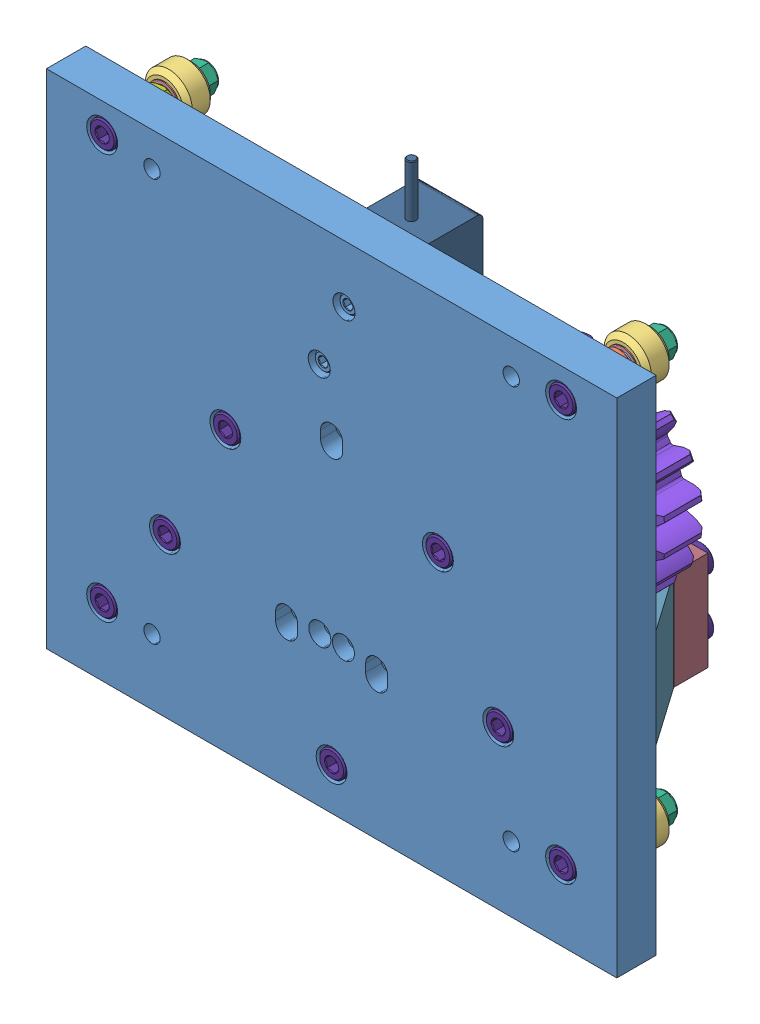
SolidWorks assembly Rudder Pedal Gantry Carriage, configuration Default. Lengths in mm.
Overall size (184.15 170.4 106.96).
90 component instances, 20 part files, 100 mates.
Components (placement in the parent):
- Rudder Pedal Gantry Interface Plate-1: Rudder Pedal Gantry Interface Plate [Default] at (90.01 5647.6627 2781.41) size (184.15 162.18 12.7)
- 819368021615 - Aluminum Spacer 6mm-1: 819368021615 - Aluminum Spacer 6mm [Default] at (74.085 5582.1627 2775.41) x (-1 0 0) z (0 0 1) size (10 10 6)
- 819368020823 - Delrin Mini V Wheel-4: 819368020823 - Delrin Mini V Wheel [Straight] at (74.085 5582.1627 2769.71) x (1 0 0) z (0 -1 0) size (15.23 15.4 15.23)
  - Delrin Mini V Wheel-1: Delrin Mini V Wheel [Default] x (0 -1 0) z (0 0 1) size (8.8 15.23 15.23)
  - Ball Bearing 5 x 10 x 4.2-1: Ball Bearing 5 x 10 x 4.2 [Default] at (0 -2.6 0) x (0 -1 0) z (0.990411 0 0.138155) size (4.2 10 10)
  - Ball Bearing 5 x 10 x 4.2-2: Ball Bearing 5 x 10 x 4.2 [Default] at (0 2.6 0) x (0 1 0) z (-0.887666 0 -0.460488) size (4.2 10 10)
  - Precision Shim 8 x 5 x 1-1: Precision Shim 8 x 5 x 1 [Default] at (0 -0.5 0) x (0.977063 0 -0.212952) z (0.212952 0 0.977063) size (8 1 8)
  - Precision Shim 8 x 5 x 1-2: Precision Shim 8 x 5 x 1 [Default] at (0 4.7 0) x (0.633048 0 -0.774113) z (0.774113 0 0.633048) size (8 1 8)
  - Nylon Insert Lock Nut M5-1: Nylon Insert Lock Nut M5 [Default] at (0 -4.7 0) x (-0.212185 0 -0.97723) z (-0.97723 0 0.212185) size (8 5 9.24)
- 819368021615 - Aluminum Spacer 6mm-2: 819368021615 - Aluminum Spacer 6mm [Default] at (74.085 5452.174 2775.41) x (-0.573309 0.819339 0) z (0 0 1) size (10 10 6)
- 819368020823 - Delrin Mini V Wheel-1: 819368020823 - Delrin Mini V Wheel [Straight] at (74.085 5452.174 2769.71) x (1 0 0) z (0 -1 0) size (15.23 15.4 15.23)
  - Delrin Mini V Wheel-1: Delrin Mini V Wheel [Default] x (0 -1 0) z (0 0 1) size (8.8 15.23 15.23)
  - Ball Bearing 5 x 10 x 4.2-1: Ball Bearing 5 x 10 x 4.2 [Default] at (0 -2.6 0) x (0 -1 0) z (0.990411 0 0.138155) size (4.2 10 10)
  - Ball Bearing 5 x 10 x 4.2-2: Ball Bearing 5 x 10 x 4.2 [Default] at (0 2.6 0) x (0 1 0) z (-0.887666 0 -0.460488) size (4.2 10 10)
  - Precision Shim 8 x 5 x 1-1: Precision Shim 8 x 5 x 1 [Default] at (0 -0.5 0) x (0.977063 0 -0.212952) z (0.212952 0 0.977063) size (8 1 8)
  - Precision Shim 8 x 5 x 1-2: Precision Shim 8 x 5 x 1 [Default] at (0 4.7 0) x (0.633048 0 -0.774113) z (0.774113 0 0.633048) size (8 1 8)
  - Nylon Insert Lock Nut M5-1: Nylon Insert Lock Nut M5 [Default] at (0 -4.7 0) x (-0.212185 0 -0.97723) z (-0.97723 0 0.212185) size (8 5 9.24)
- 819368021011 - Eccentric Spacer 6mm-1: 819368021011 - Eccentric Spacer 6mm [Default] at (-73.351 5581.8705 2781.41) x (0.369816 0.929105 0) z (-0.929105 0.369816 0) size (11.55 8.5 10)
- 819368020823 - Delrin Mini V Wheel-2: 819368020823 - Delrin Mini V Wheel [Straight] at (-74.085 5582.1627 2769.71) x (-1 0 0) z (0 1 0) size (15.23 15.4 15.23)
  - Delrin Mini V Wheel-1: Delrin Mini V Wheel [Default] x (0 -1 0) z (0 0 1) size (8.8 15.23 15.23)
  - Ball Bearing 5 x 10 x 4.2-1: Ball Bearing 5 x 10 x 4.2 [Default] at (0 -2.6 0) x (0 -1 0) z (0.990411 0 0.138155) size (4.2 10 10)
  - Ball Bearing 5 x 10 x 4.2-2: Ball Bearing 5 x 10 x 4.2 [Default] at (0 2.6 0) x (0 1 0) z (-0.887666 0 -0.460488) size (4.2 10 10)
  - Precision Shim 8 x 5 x 1-1: Precision Shim 8 x 5 x 1 [Default] at (0 -0.5 0) x (0.977063 0 -0.212952) z (0.212952 0 0.977063) size (8 1 8)
  - Precision Shim 8 x 5 x 1-2: Precision Shim 8 x 5 x 1 [Default] at (0 4.7 0) x (0.633048 0 -0.774113) z (0.774113 0 0.633048) size (8 1 8)
  - Nylon Insert Lock Nut M5-1: Nylon Insert Lock Nut M5 [Default] at (0 -4.7 0) x (-0.212185 0 -0.97723) z (-0.97723 0 0.212185) size (8 5 9.24)
- 819368021011 - Eccentric Spacer 6mm-2: 819368021011 - Eccentric Spacer 6mm [Default] at (-74.085 5452.174 2781.41) x (-1 0 0) z (0 -1 0) size (11.55 8.5 10)
- 819368020823 - Delrin Mini V Wheel-3: 819368020823 - Delrin Mini V Wheel [Straight] at (-74.085 5452.174 2769.71) x (-1 0 0) z (0 1 0) size (15.23 15.4 15.23)
  - Delrin Mini V Wheel-1: Delrin Mini V Wheel [Default] x (0 -1 0) z (0 0 1) size (8.8 15.23 15.23)
  - Ball Bearing 5 x 10 x 4.2-1: Ball Bearing 5 x 10 x 4.2 [Default] at (0 -2.6 0) x (0 -1 0) z (0.990411 0 0.138155) size (4.2 10 10)
  - Ball Bearing 5 x 10 x 4.2-2: Ball Bearing 5 x 10 x 4.2 [Default] at (0 2.6 0) x (0 1 0) z (-0.887666 0 -0.460488) size (4.2 10 10)
  - Precision Shim 8 x 5 x 1-1: Precision Shim 8 x 5 x 1 [Default] at (0 -0.5 0) x (0.977063 0 -0.212952) z (0.212952 0 0.977063) size (8 1 8)
  - Precision Shim 8 x 5 x 1-2: Precision Shim 8 x 5 x 1 [Default] at (0 4.7 0) x (0.633048 0 -0.774113) z (0.774113 0 0.633048) size (8 1 8)
  - Nylon Insert Lock Nut M5-1: Nylon Insert Lock Nut M5 [Default] at (0 -4.7 0) x (-0.212185 0 -0.97723) z (-0.97723 0 0.212185) size (8 5 9.24)
- GEAR, 3M x 20T x 20PA x 5mm Bore-1: GEAR, 3M x 20T x 20PA x 5mm Bore [Metric - Spur gear 3M 20T 20PA 13FW ---S20O75H20L7N] at (34.31 5519.674 2753.66) x (0 0 -1) z (1 0 0) size (40.75 65.41 65.41)
- GEAR, 3M x 20T x 20PA x 5mm Bore-2: GEAR, 3M x 20T x 20PA x 5mm Bore [Metric - Spur gear 3M 20T 20PA 13FW ---S20O75H20L7N] at (-34.31 5519.674 2753.66) x (0 0 -1) z (1 0 0) size (40.75 65.41 65.41)
- Rudder Pedal Gantry Locking Arm-1: Rudder Pedal Gantry Locking Arm [Default] at (-40.8902 5534.6112 2781.4126) size (85.77 81.54 25.4)
- B14HDP-254-B-4-1: B14HDP-254-B-4 [Default] at (8.6106 5583.123 2781.4126) x (0 0 1) z (0 -1 0) size (26.15 43.85 56.44)
- 1692K230 - SPRING, COMPRESSION, CONFINED SPACE, .60 OD x .625L x 3.57lbs RATE-1: 1692K230 - SPRING, COMPRESSION, CONFINED SPACE, .60 OD x .625L x 3.57lbs RATE [1692K23] at (0 5480.9876 2772.5226) x (0.468976 0 -0.883211) z (0.883211 0 0.468976) size (14.74 6.35 14.56)
- Rudder Pedal Gantry Locking Arm Spring Stop-1: Rudder Pedal Gantry Locking Arm Spring Stop [Default] at (-0.8374 5480.9876 2772.2543) x (-1 0 0) z (0 1 0) size (13.72 15.75 8.89)
- Rudder Carriage Linear Bearing Holder-1: Rudder Carriage Linear Bearing Holder [Default] at (339.725 -1087.7493 -123.7365) size (123.48 58.99 94.03)
  - Rudder Carriage Linear Bearing Holder Lower Shell-1: Rudder Carriage Linear Bearing Holder Lower Shell [Default] at origin size (40 32 10.95)
  - Rudder Carriage Linear Bearing Holder Upper Shell-1: Rudder Carriage Linear Bearing Holder Upper Shell [Default] at origin size (123.48 58.99 77.75)
  - LM8UU v2-1: LM8UU v2 [Default] at (-339.725 6533.262 2827.3504) size (14.96 23.84 14.96)
  - 93625A200 - NUT, M5-0.8, NYLOC, 18-8-1: 93625A200 - NUT, M5-0.8, NYLOC, 18-8 [93625A200] at (-326.725 6524.262 2838.3504) x (-1 0 0) z (0 1 0) size (8 5.15 9.24)
  - 93705A838 - SHCS, M5-0.8 x 30mm, SELF-LOCKING, 18-8-1: 93705A838 - SHCS, M5-0.8 x 30mm, SELF-LOCKING, 18-8 [91292A194] at (-326.725 6524.262 2846.3504) x (0.267759 0.963486 0) z (0 0 1) size (8.5 8.5 35.49)
  - 93625A200 - NUT, M5-0.8, NYLOC, 18-8-2: 93625A200 - NUT, M5-0.8, NYLOC, 18-8 [93625A200] at (-352.725 6524.262 2838.3504) x (-1 0 0) z (0 1 0) size (8 5.15 9.24)
  - 93705A838 - SHCS, M5-0.8 x 30mm, SELF-LOCKING, 18-8-2: 93705A838 - SHCS, M5-0.8 x 30mm, SELF-LOCKING, 18-8 [91292A194] at (-352.725 6524.262 2846.3504) x (0.111609 0.993752 0) z (0 0 1) size (8.5 8.5 35.49)
  - 93625A200 - NUT, M5-0.8, NYLOC, 18-8-3: 93625A200 - NUT, M5-0.8, NYLOC, 18-8 [93625A200] at (-326.725 6542.262 2838.3504) x (-1 0 0) z (0 1 0) size (8 5.15 9.24)
  - 93705A838 - SHCS, M5-0.8 x 30mm, SELF-LOCKING, 18-8-3: 93705A838 - SHCS, M5-0.8 x 30mm, SELF-LOCKING, 18-8 [91292A194] at (-326.725 6542.262 2846.3504) x (-0.015836 0.999875 0) z (0 0 1) size (8.5 8.5 35.49)
  - 93625A200 - NUT, M5-0.8, NYLOC, 18-8-4: 93625A200 - NUT, M5-0.8, NYLOC, 18-8 [93625A200] at (-352.725 6542.262 2838.3504) x (-1 0 0) z (0 1 0) size (8 5.15 9.24)
  - 93705A838 - SHCS, M5-0.8 x 30mm, SELF-LOCKING, 18-8-4: 93705A838 - SHCS, M5-0.8 x 30mm, SELF-LOCKING, 18-8 [91292A194] at (-352.725 6542.262 2846.3504) x (-0.108968 0.994045 0) z (0 0 1) size (8.5 8.5 35.49)
- 93705A838 - SHCS, M5-0.8 x 30mm, SELF-LOCKING, 18-8-1: 93705A838 - SHCS, M5-0.8 x 30mm, SELF-LOCKING, 18-8 [91292A194] at (-34.31 5496.9376 2768.7126) x (-1 0 0.000529) z (0 1 0) size (8.5 8.5 35.49)
- 93625A200 - NUT, M5-0.8, NYLOC, 18-8-1: 93625A200 - NUT, M5-0.8, NYLOC, 18-8 [93625A200] at (-34.31 5478.9696 2768.7126) x (0.99571 0 -0.092533) z (0.092533 0 0.99571) size (8 5.15 9.24)
- 90126A029 - WASHER, .25 x .625, STEEL, ZINC-1: 90126A029 - WASHER, .25 x .625, STEEL, ZINC [90126A029] at (-34.31 5478.9696 2768.7126) x (0 -1 0) z (-0.092533 0 -0.99571) size (2.03 15.88 15.88)
- 93705A838 - SHCS, M5-0.8 x 30mm, SELF-LOCKING, 18-8-2: 93705A838 - SHCS, M5-0.8 x 30mm, SELF-LOCKING, 18-8 [91292A194] at (34.31 5496.9376 2768.7126) x (0.981982 0 -0.188974) z (0 1 0) size (8.5 8.5 35.49)
- 93625A200 - NUT, M5-0.8, NYLOC, 18-8-2: 93625A200 - NUT, M5-0.8, NYLOC, 18-8 [93625A200] at (34.31 5478.9696 2768.7126) x (-0.982082 0 0.188455) z (-0.188455 0 -0.982082) size (8 5.15 9.24)
- 90126A029 - WASHER, .25 x .625, STEEL, ZINC-2: 90126A029 - WASHER, .25 x .625, STEEL, ZINC [90126A029] at (34.31 5478.9696 2768.7126) x (0 -1 0) z (0.188455 0 0.982082) size (2.03 15.88 15.88)
- 93705A838 - SHCS, M5-0.8 x 30mm, SELF-LOCKING, 18-8-3: 93705A838 - SHCS, M5-0.8 x 30mm, SELF-LOCKING, 18-8 [91292A194] at (-34.31 5519.674 2759.11) x (-1 0.000529 0) z (0 0 -1) size (8.5 8.5 35.49)
- 93625A200 - NUT, M5-0.8, NYLOC, 18-8-3: 93625A200 - NUT, M5-0.8, NYLOC, 18-8 [93625A200] at (-34.31 5519.674 2765.11) x (0.973495 -0.228707 0) z (0.228707 0.973495 0) size (8 5.15 9.24)
- 90126A029 - WASHER, .25 x .625, STEEL, ZINC-3: 90126A029 - WASHER, .25 x .625, STEEL, ZINC [90126A029] at (-34.31 5519.674 2767.142) x (0 0 -1) z (-0.092533 0.99571 0) size (2.03 15.88 15.88)
- 93705A838 - SHCS, M5-0.8 x 30mm, SELF-LOCKING, 18-8-4: 93705A838 - SHCS, M5-0.8 x 30mm, SELF-LOCKING, 18-8 [91292A194] at (34.31 5519.674 2759.11) x (-0.987434 -0.158031 0) z (0 0 -1) size (8.5 8.5 35.49)
- 93625A200 - NUT, M5-0.8, NYLOC, 18-8-4: 93625A200 - NUT, M5-0.8, NYLOC, 18-8 [93625A200] at (34.31 5519.674 2765.11) x (0.997443 -0.071464 0) z (0.071464 0.997443 0) size (8 5.15 9.24)
- 90126A029 - WASHER, .25 x .625, STEEL, ZINC-4: 90126A029 - WASHER, .25 x .625, STEEL, ZINC [90126A029] at (34.31 5519.674 2767.142) x (0 0 -1) z (-0.249235 0.968443 0) size (2.03 15.88 15.88)
- Ball Bearing 5 x 10 x 4.2-1: Ball Bearing 5 x 10 x 4.2 [Default] at (34.31 5519.674 2778.5139) x (0 0 1) z (-0.998847 0.048007 0) size (4.2 10 10)
- Ball Bearing 5 x 10 x 4.2-2: Ball Bearing 5 x 10 x 4.2 [Default] at (-34.31 5519.674 2778.5139) x (0 0 1) z (-0.617174 -0.786826 0) size (4.2 10 10)
- 93705A838 - SHCS, M5-0.8 x 30mm, SELF-LOCKING, 18-8-6: 93705A838 - SHCS, M5-0.8 x 30mm, SELF-LOCKING, 18-8 [91292A194] at (-53.8009 5480.5627 2759.11) x (0.987434 0.158031 0) z (0 0 -1) size (8.5 8.5 35.49)
- 90126A029 - WASHER, .25 x .625, STEEL, ZINC-6: 90126A029 - WASHER, .25 x .625, STEEL, ZINC [90126A029] at (-53.8009 5480.5627 2771.885) x (0 0 -1) z (0.249235 -0.968443 0) size (2.03 15.88 15.88)
- 93625A200 - NUT, M5-0.8, NYLOC, 18-8-6: 93625A200 - NUT, M5-0.8, NYLOC, 18-8 [93625A200] at (-53.8009 5480.5627 2769.853) x (-0.99742 0.071781 0) z (-0.071781 -0.99742 0) size (8 5.15 9.24)
- 93705A838 - SHCS, M5-0.8 x 30mm, SELF-LOCKING, 18-8-7: 93705A838 - SHCS, M5-0.8 x 30mm, SELF-LOCKING, 18-8 [91292A194] at (0 5443.1314 2759.11) x (0.949887 0.312592 0) z (0 0 -1) size (8.5 8.5 35.49)
- 90126A029 - WASHER, .25 x .625, STEEL, ZINC-7: 90126A029 - WASHER, .25 x .625, STEEL, ZINC [90126A029] at (0 5443.1314 2771.885) x (0 0 -1) z (0.399631 -0.916676 0) size (2.03 15.88 15.88)
- 93625A200 - NUT, M5-0.8, NYLOC, 18-8-7: 93625A200 - NUT, M5-0.8, NYLOC, 18-8 [93625A200] at (0 5443.1314 2769.853) x (-0.996185 -0.087271 0) z (0.087271 -0.996185 0) size (8 5.15 9.24)
- 93705A838 - SHCS, M5-0.8 x 30mm, SELF-LOCKING, 18-8-9: 93705A838 - SHCS, M5-0.8 x 30mm, SELF-LOCKING, 18-8 [91292A194] at (53.8009 5480.5627 2759.11) x (0.902352 0.430999 0) z (0 0 -1) size (8.5 8.5 35.49)
- 90126A029 - WASHER, .25 x .625, STEEL, ZINC-9: 90126A029 - WASHER, .25 x .625, STEEL, ZINC [90126A029] at (53.8009 5480.5627 2771.885) x (0 0 -1) z (0.513101 -0.858328 0) size (2.03 15.88 15.88)
- 93625A200 - NUT, M5-0.8, NYLOC, 18-8-9: 93625A200 - NUT, M5-0.8, NYLOC, 18-8 [93625A200] at (53.8009 5480.5627 2769.853) x (-0.976963 -0.213407 0) z (0.213407 -0.976963 0) size (8 5.15 9.24)
- 93705A838 - SHCS, M5-0.8 x 30mm, SELF-LOCKING, 18-8-11: 93705A838 - SHCS, M5-0.8 x 30mm, SELF-LOCKING, 18-8 [91292A194] at (-74.085 5582.1627 2759.11) x (0.902352 0.430999 0) z (0 0 -1) size (8.5 8.5 35.49)
- 93705A838 - SHCS, M5-0.8 x 30mm, SELF-LOCKING, 18-8-12: 93705A838 - SHCS, M5-0.8 x 30mm, SELF-LOCKING, 18-8 [91292A194] at (-74.085 5451.384 2759.11) x (0.822602 0.568618 0) z (0 0 -1) size (8.5 8.5 35.49)
- 93705A838 - SHCS, M5-0.8 x 30mm, SELF-LOCKING, 18-8-14: 93705A838 - SHCS, M5-0.8 x 30mm, SELF-LOCKING, 18-8 [91292A194] at (74.085 5452.174 2759.11) x (0.743503 0.668733 0) z (0 0 -1) size (8.5 8.5 35.49)
- 93705A838 - SHCS, M5-0.8 x 30mm, SELF-LOCKING, 18-8-16: 93705A838 - SHCS, M5-0.8 x 30mm, SELF-LOCKING, 18-8 [91292A194] at (74.085 5582.1627 2759.11) x (0.677932 0.735125 0) z (0 0 -1) size (8.5 8.5 35.49)
- 91251A146 - SHCS, 6-32 X .375, STEEL, BLACK-OXIDE-1: 91251A146 - SHCS, 6-32 X .375, STEEL, BLACK-OXIDE [91251A146] at (4 5573.123 2779.8098) x (0.923728 0.383049 0) z (0 0 -1) size (5.74 5.74 13.47)
- 91251A146 - SHCS, 6-32 X .375, STEEL, BLACK-OXIDE-2: 91251A146 - SHCS, 6-32 X .375, STEEL, BLACK-OXIDE [91251A146] at (-4 5553.123 2779.8098) x (0.923728 0.383049 0) z (0 0 -1) size (5.74 5.74 13.47)
- 91251A146 - SHCS, 6-32 X .375, STEEL, BLACK-OXIDE-3: 91251A146 - SHCS, 6-32 X .375, STEEL, BLACK-OXIDE [91251A146] at (-3.81 5477.8126 2777.2698) x (0.923728 0.383049 0) z (0 0 -1) size (5.74 5.74 13.47)
- 91251A146 - SHCS, 6-32 X .375, STEEL, BLACK-OXIDE-4: 91251A146 - SHCS, 6-32 X .375, STEEL, BLACK-OXIDE [91251A146] at (3.81 5477.8126 2777.2698) x (0.923728 0.383049 0) z (0 0 -1) size (5.74 5.74 13.47)
- 91251A146 - SHCS, 6-32 X .375, STEEL, BLACK-OXIDE-5: 91251A146 - SHCS, 6-32 X .375, STEEL, BLACK-OXIDE [91251A146] at (-14.5414 5476.9439 2777.2698) x (0.216826 -0.97621 0) z (0 0 -1) size (5.74 5.74 13.47)
- 91251A146 - SHCS, 6-32 X .375, STEEL, BLACK-OXIDE-7: 91251A146 - SHCS, 6-32 X .375, STEEL, BLACK-OXIDE [91251A146] at (14.5414 5476.9439 2777.2698) x (0.044015 -0.999031 0) z (0 0 -1) size (5.74 5.74 13.47)
- 91251A146 - SHCS, 6-32 X .375, STEEL, BLACK-OXIDE-9: 91251A146 - SHCS, 6-32 X .375, STEEL, BLACK-OXIDE [91251A146] at (0 5534.964 2777.2698) x (-0.130134 -0.991496 0) z (0 0 -1) size (5.74 5.74 13.47)
- 93365A130 - INSERT, 6-32, BRASS, FOR PLASTICS-2: 93365A130 - INSERT, 6-32, BRASS, FOR PLASTICS [93365A130] at (-14.5414 5476.9439 2781.4126) x (-0.85131 -0.524663 0) z (-0.524663 0.85131 0) size (5.56 4.29 5.56)
- 93365A130 - INSERT, 6-32, BRASS, FOR PLASTICS-4: 93365A130 - INSERT, 6-32, BRASS, FOR PLASTICS [93365A130] at (14.5414 5476.9439 2781.4126) x (-0.777574 -0.628792 0) z (-0.628792 0.777574 0) size (5.56 4.29 5.56)
- 93365A130 - INSERT, 6-32, BRASS, FOR PLASTICS-6: 93365A130 - INSERT, 6-32, BRASS, FOR PLASTICS [93365A130] at (-3.81 5477.8126 2781.4126) x (-0.715577 -0.698533 0) z (-0.698533 0.715577 0) size (5.56 4.29 5.56)
- 93365A130 - INSERT, 6-32, BRASS, FOR PLASTICS-8: 93365A130 - INSERT, 6-32, BRASS, FOR PLASTICS [93365A130] at (3.81 5477.8126 2781.4126) x (-0.676489 -0.736453 0) z (-0.736453 0.676489 0) size (5.56 4.29 5.56)
- 93365A130 - INSERT, 6-32, BRASS, FOR PLASTICS-1: 93365A130 - INSERT, 6-32, BRASS, FOR PLASTICS [93365A130] at (0 5534.964 2781.4126) x (-0.923728 -0.383049 0) z (-0.383049 0.923728 0) size (5.56 4.29 5.56)
Mates (geometry in assembly coordinates):
- Concentric67: concentric: cylinder of 819368020823 - Delrin Mini V Wheel-4/Precision Shim 8 x 5 x 1-2 through (74.085 5582.1627 2775.41) axis (0 0 -1) radius 4; cylinder of 819368021615 - Aluminum Spacer 6mm-1 through (74.085 5582.1627 2781.41) axis (0 0 -1) radius 5
- Coincident356: coincident: plane of 819368020823 - Delrin Mini V Wheel-4/Precision Shim 8 x 5 x 1-2 through (74.085 5582.1627 2775.41) normal (0 0 1); plane of 819368021615 - Aluminum Spacer 6mm-1 through (74.085 5582.1627 2775.41) normal (0 0 -1)
- Coincident358: coincident: plane of Rudder Pedal Gantry Interface Plate-1 through (90.01 5647.6627 2781.41) normal (0 0 -1); plane of 819368021615 - Aluminum Spacer 6mm-1 through (74.085 5582.1627 2781.41) normal (0 0 1)
- Distance9: distance = 9.525 mm: plane of 819368021615 - Aluminum Spacer 6mm-1 through (74.085 5582.1627 2775.41) normal (0 -1 0); plane of Rudder Pedal Gantry Interface Plate-1 through (92.075 5591.6877 2794.11) normal (0 1 0)
- Coincident359: coincident: plane of 819368020823 - Delrin Mini V Wheel-4 through (74.085 5582.1627 2769.71) normal (0 0 1); plane of 819368020823 - Delrin Mini V Wheel-1 through (74.085 5452.174 2769.71) normal (0 0 1)
- Coincident360: coincident: plane of 819368020823 - Delrin Mini V Wheel-4 through (74.085 5582.1627 2769.71) normal (1 0 0); plane of 819368020823 - Delrin Mini V Wheel-1 through (74.085 5452.174 2769.71) normal (1 0 0)
- Concentric68: concentric: cylinder of 819368020823 - Delrin Mini V Wheel-1/Precision Shim 8 x 5 x 1-2 through (74.085 5452.174 2775.41) axis (0 0 -1) radius 4; cylinder of 819368021615 - Aluminum Spacer 6mm-2 through (74.085 5452.174 2781.41) axis (0 0 -1) radius 5
- Coincident361: coincident: plane of 819368020823 - Delrin Mini V Wheel-1/Precision Shim 8 x 5 x 1-2 through (74.085 5452.174 2775.41) normal (0 0 1); plane of 819368021615 - Aluminum Spacer 6mm-2 through (74.085 5452.174 2775.41) normal (0 0 -1)
- Concentric70: concentric aligned: cylinder of 819368020823 - Delrin Mini V Wheel-2/Precision Shim 8 x 5 x 1-2 through (-74.085 5582.1627 2775.41) axis (0 0 -1) radius 4; cylinder of 819368021011 - Eccentric Spacer 6mm-1 through (-74.085 5582.1627 2783.91) axis (0 0 -1) radius 2.5
- Coincident362: coincident anti-aligned: plane of 819368020823 - Delrin Mini V Wheel-2/Precision Shim 8 x 5 x 1-2 through (-74.085 5582.1627 2775.41) normal (0 0 1); circle of 819368021011 - Eccentric Spacer 6mm-1
- Concentric71: concentric aligned: cylinder of 819368020823 - Delrin Mini V Wheel-3/Delrin Mini V Wheel-1 through (-74.085 5452.174 2769.71) axis (0 0 -1) radius 7.615; cylinder of 819368021011 - Eccentric Spacer 6mm-2 through (-74.085 5452.174 2783.91) axis (0 0 -1) radius 3.555
- Coincident363: coincident anti-aligned: plane of 819368020823 - Delrin Mini V Wheel-3/Precision Shim 8 x 5 x 1-2 through (-74.085 5452.174 2775.41) normal (0 0 1); circle of 819368021011 - Eccentric Spacer 6mm-2
- Parallel3: parallel aligned: plane of GEAR, 3M x 20T x 20PA x 5mm Bore-1 through (34.31 5519.674 2781.4139) normal (0 0 1); plane of Rudder Pedal Gantry Locking Arm-1 through (-40.8902 5534.6112 2781.4126) normal (0 0 1)
- Coincident414: coincident: cone of GEAR, 3M x 20T x 20PA x 5mm Bore-2 through (-34.31 5497.235 2768.7139) axis (0 1 0); circle of 93705A838 - SHCS, M5-0.8 x 30mm, SELF-LOCKING, 18-8-1
- Tangent18: tangent anti-aligned: cylinder of GEAR, 3M x 20T x 20PA x 5mm Bore-2 through (-34.31 5519.674 2781.4139) axis (0 0 -1) radius 26.249; plane of B14HDP-254-B-4-1 through (10 5545.923 2757.2626) normal (0 -1 0)
- Concentric82: concentric anti-aligned: cylinder of Rudder Pedal Gantry Locking Arm-1 through (-34.31 5461.9376 2768.7126) axis (0 -1 0) radius 2.75; cylinder of 93705A838 - SHCS, M5-0.8 x 30mm, SELF-LOCKING, 18-8-1 through (-34.31 5466.9376 2768.7126) axis (0 1 0) radius 2.5
- Coincident405: coincident anti-aligned: plane of Rudder Pedal Gantry Locking Arm-1 through (-31.56 5466.9376 2768.7126) normal (0 -1 0); plane of 93705A838 - SHCS, M5-0.8 x 30mm, SELF-LOCKING, 18-8-1 through (-34.31 5466.9376 2768.7126) normal (0 1 0)
- Coincident406: coincident: plane of assembly; plane of Rudder Pedal Gantry Locking Arm-1 through (50.8 5476.9376 2756.0126) normal (0 1 0); plane of 90126A029 - WASHER, .25 x .625, STEEL, ZINC-1 through (-34.31 5476.9376 2768.7126) normal (0 -1 0)
- Concentric87: concentric anti-aligned: cylinder of Rudder Pedal Gantry Locking Arm-1 through (34.31 5461.9376 2768.7126) axis (0 -1 0) radius 2.75; cylinder of 93705A838 - SHCS, M5-0.8 x 30mm, SELF-LOCKING, 18-8-2 through (34.31 5466.9376 2768.7126) axis (0 1 0) radius 2.5
- Coincident409: coincident anti-aligned: plane of Rudder Pedal Gantry Locking Arm-1 through (37.06 5466.9376 2768.7126) normal (0 -1 0); plane of 93705A838 - SHCS, M5-0.8 x 30mm, SELF-LOCKING, 18-8-2 through (34.31 5466.9376 2768.7126) normal (0 1 0)
- Coincident410: coincident: plane of assembly; plane of Rudder Pedal Gantry Locking Arm-1 through (50.8 5476.9376 2756.0126) normal (0 1 0); plane of 90126A029 - WASHER, .25 x .625, STEEL, ZINC-2 through (34.31 5476.9376 2768.7126) normal (0 -1 0)
- Coincident418: coincident anti-aligned: plane of Rudder Pedal Gantry Locking Arm-1 through (0 5487.3376 2790.3026) normal (0 -1 0); plane of 1692K230 - SPRING, COMPRESSION, CONFINED SPACE, .60 OD x .625L x 3.57lbs RATE-1 through (0 5487.3376 2772.5226) normal (0 1 0)
- Concentric93: concentric anti-aligned: cylinder of Rudder Pedal Gantry Locking Arm-1 through (0 5487.3376 2772.5226) axis (0 -1 0) radius 7.62; circle of 1692K230 - SPRING, COMPRESSION, CONFINED SPACE, .60 OD x .625L x 3.57lbs RATE-1
- Coincident425: coincident aligned: plane of Rudder Pedal Gantry Locking Arm-1 through (-40.8902 5534.6112 2781.4126) normal (0 0 1); plane of Rudder Pedal Gantry Locking Arm Spring Stop-1 through (-6.858 5447.4039 2781.4126) normal (0 0 1)
- Width4: width anti-aligned: plane of Rudder Pedal Gantry Locking Arm Spring Stop-1 through (-6.858 5447.4039 2772.5226) normal (-1 0 0); plane of Rudder Pedal Gantry Locking Arm-1 through (6.858 5447.4039 2781.4126) normal (1 0 0); plane of Rudder Pedal Gantry Locking Arm Spring Stop-1 through (-7.62 5487.3376 2790.3026) normal (1 0 0); plane of Rudder Pedal Gantry Locking Arm-1 through (7.62 5487.3376 2790.3026) normal (-1 0 0)
- Concentric83: concentric anti-aligned: circle of 93705A838 - SHCS, M5-0.8 x 30mm, SELF-LOCKING, 18-8-1; circle of 93625A200 - NUT, M5-0.8, NYLOC, 18-8-1
- Concentric84: concentric anti-aligned: circle of 93625A200 - NUT, M5-0.8, NYLOC, 18-8-1; cylinder of 90126A029 - WASHER, .25 x .625, STEEL, ZINC-1 through (-34.31 5476.9376 2768.7126) axis (0 1 0) radius 7.9375
- Coincident407: coincident anti-aligned: plane of 93625A200 - NUT, M5-0.8, NYLOC, 18-8-1 through (-34.7374 5478.9696 2764.1137) normal (0 -1 0); plane of 90126A029 - WASHER, .25 x .625, STEEL, ZINC-1 through (-34.31 5478.9696 2768.7126) normal (0 1 0)
- Concentric85: concentric anti-aligned: circle of 93705A838 - SHCS, M5-0.8 x 30mm, SELF-LOCKING, 18-8-2; circle of 93625A200 - NUT, M5-0.8, NYLOC, 18-8-2
- Concentric86: concentric anti-aligned: circle of 93625A200 - NUT, M5-0.8, NYLOC, 18-8-2; cylinder of 90126A029 - WASHER, .25 x .625, STEEL, ZINC-2 through (34.31 5476.9376 2768.7126) axis (0 1 0) radius 7.9375
- Coincident408: coincident anti-aligned: plane of 93625A200 - NUT, M5-0.8, NYLOC, 18-8-2 through (35.1804 5478.9696 2773.2487) normal (0 -1 0); plane of 90126A029 - WASHER, .25 x .625, STEEL, ZINC-2 through (34.31 5478.9696 2768.7126) normal (0 1 0)
- Coincident426: coincident aligned: plane of 1692K230 - SPRING, COMPRESSION, CONFINED SPACE, .60 OD x .625L x 3.57lbs RATE-1 through (0 5480.9876 2772.5226) normal (0 1 0); plane of Rudder Pedal Gantry Locking Arm Spring Stop-1 through (0 5480.9876 2772.5226) normal (0 1 0)
- Parallel5: parallel: plane of Rudder Pedal Gantry Interface Plate-1 through (90.01 5647.6627 2781.41) normal (0 0 -1); plane of ? through (0 5445.5127 2714.6139) normal (0 0 1)
- Coincident445: coincident: plane of Rudder Pedal Gantry Interface Plate-1 through (20 5429.5127 2703.6139) normal (0 -1 0); plane of Rudder Carriage Linear Bearing Holder-1/Rudder Carriage Linear Bearing Holder Upper Shell-1 through (20 5429.5127 2703.6139) normal (0 -1 0)
- Concentric94: concentric: cylinder of Rudder Pedal Gantry Interface Plate-1 through (-34.31 5519.674 2794.11) axis (0 0 1) radius 5; cylinder of 93705A838 - SHCS, M5-0.8 x 30mm, SELF-LOCKING, 18-8-3 through (-34.31 5519.674 2789.11) axis (0 0 -1) radius 2.5
- Coincident446: coincident: plane of Rudder Pedal Gantry Interface Plate-1 through (-31.41 5519.674 2789.11) normal (0 0 1); plane of 93705A838 - SHCS, M5-0.8 x 30mm, SELF-LOCKING, 18-8-3 through (-34.31 5519.674 2789.11) normal (0 0 -1)
- Concentric95: concentric anti-aligned: cylinder of 93705A838 - SHCS, M5-0.8 x 30mm, SELF-LOCKING, 18-8-3 through (-34.31 5519.674 2794.11) axis (0 0 -1) radius 4.25; circle of 93625A200 - NUT, M5-0.8, NYLOC, 18-8-3
- Distance10: distance = 1 mm aligned: plane of 93625A200 - NUT, M5-0.8, NYLOC, 18-8-3 through (-35.3664 5515.1776 2760.11) normal (0 0 -1); plane of 93705A838 - SHCS, M5-0.8 x 30mm, SELF-LOCKING, 18-8-3 through (-34.31 5519.674 2759.11) normal (0 0 -1)
- Concentric96: concentric anti-aligned: circle of 93705A838 - SHCS, M5-0.8 x 30mm, SELF-LOCKING, 18-8-3; cylinder of 90126A029 - WASHER, .25 x .625, STEEL, ZINC-3 through (-34.31 5519.674 2765.11) axis (0 0 1) radius 7.9375
- Coincident447: coincident anti-aligned: plane of 93625A200 - NUT, M5-0.8, NYLOC, 18-8-3 through (-35.3664 5515.1776 2765.11) normal (0 0 1); plane of 90126A029 - WASHER, .25 x .625, STEEL, ZINC-3 through (-34.31 5519.674 2765.11) normal (0 0 -1)
- Concentric97: concentric anti-aligned: cylinder of 93705A838 - SHCS, M5-0.8 x 30mm, SELF-LOCKING, 18-8-4 through (34.31 5519.674 2794.11) axis (0 0 -1) radius 4.25; circle of 93625A200 - NUT, M5-0.8, NYLOC, 18-8-4
- Distance11: distance = 1 mm aligned: plane of 93625A200 - NUT, M5-0.8, NYLOC, 18-8-4 through (33.9799 5515.067 2760.11) normal (0 0 -1); plane of 93705A838 - SHCS, M5-0.8 x 30mm, SELF-LOCKING, 18-8-4 through (34.31 5519.674 2759.11) normal (0 0 -1)
- Concentric98: concentric anti-aligned: circle of 93705A838 - SHCS, M5-0.8 x 30mm, SELF-LOCKING, 18-8-4; cylinder of 90126A029 - WASHER, .25 x .625, STEEL, ZINC-4 through (34.31 5519.674 2765.11) axis (0 0 1) radius 7.9375
- Coincident448: coincident anti-aligned: plane of 93625A200 - NUT, M5-0.8, NYLOC, 18-8-4 through (33.9799 5515.067 2765.11) normal (0 0 1); plane of 90126A029 - WASHER, .25 x .625, STEEL, ZINC-4 through (34.31 5519.674 2765.11) normal (0 0 -1)
- Concentric99: concentric: cylinder of Rudder Pedal Gantry Interface Plate-1 through (34.31 5519.674 2794.11) axis (0 0 1) radius 2.9; cylinder of 93705A838 - SHCS, M5-0.8 x 30mm, SELF-LOCKING, 18-8-4 through (34.31 5519.674 2789.11) axis (0 0 -1) radius 2.5
- Coincident449: coincident: plane of Rudder Pedal Gantry Interface Plate-1 through (37.21 5519.674 2789.11) normal (0 0 1); plane of 93705A838 - SHCS, M5-0.8 x 30mm, SELF-LOCKING, 18-8-4 through (34.31 5519.674 2789.11) normal (0 0 -1)
- Concentric102: concentric aligned: cylinder of GEAR, 3M x 20T x 20PA x 5mm Bore-1 through (34.31 5519.674 2776.4139) axis (0 0 1) radius 5; cylinder of Ball Bearing 5 x 10 x 4.2-1 through (34.31 5519.674 2778.5139) axis (0 0 1) radius 5
- Coincident451: coincident anti-aligned: plane of GEAR, 3M x 20T x 20PA x 5mm Bore-1 through (34.31 5519.674 2776.4139) normal (0 0 1); plane of Ball Bearing 5 x 10 x 4.2-1 through (34.5308 5524.2687 2776.4139) normal (0 0 -1)
- Concentric103: concentric aligned: cylinder of GEAR, 3M x 20T x 20PA x 5mm Bore-2 through (-34.31 5519.674 2776.4139) axis (0 0 1) radius 5; cylinder of Ball Bearing 5 x 10 x 4.2-2 through (-34.31 5519.674 2778.5139) axis (0 0 1) radius 5
- Coincident452: coincident anti-aligned: plane of GEAR, 3M x 20T x 20PA x 5mm Bore-2 through (-34.31 5519.674 2776.4139) normal (0 0 1); plane of Ball Bearing 5 x 10 x 4.2-2 through (-37.9294 5522.513 2776.4139) normal (0 0 -1)
- Concentric104: concentric anti-aligned: cylinder of Rudder Pedal Gantry Interface Plate-1 through (-53.8009 5480.5627 2794.11) axis (0 0 1) radius 5; cylinder of 93705A838 - SHCS, M5-0.8 x 30mm, SELF-LOCKING, 18-8-6 through (-53.8009 5480.5627 2794.11) axis (0 0 -1) radius 4.25
- Coincident453: coincident anti-aligned: plane of Rudder Pedal Gantry Interface Plate-1 through (-50.9009 5480.5627 2789.11) normal (0 0 1); plane of 93705A838 - SHCS, M5-0.8 x 30mm, SELF-LOCKING, 18-8-6 through (-53.8009 5480.5627 2789.11) normal (0 0 -1)
- Concentric105: concentric anti-aligned: circle of 93705A838 - SHCS, M5-0.8 x 30mm, SELF-LOCKING, 18-8-6; cylinder of 90126A029 - WASHER, .25 x .625, STEEL, ZINC-6 through (-53.8009 5480.5627 2769.853) axis (0 0 1) radius 7.9375
- Coincident454: coincident anti-aligned: plane of Rudder Carriage Linear Bearing Holder-1/Rudder Carriage Linear Bearing Holder Upper Shell-1 through (-45.8634 5461.5127 2771.885) normal (0 0 -1); plane of 90126A029 - WASHER, .25 x .625, STEEL, ZINC-6 through (-53.8009 5480.5627 2771.885) normal (0 0 1)
- Concentric106: concentric aligned: cylinder of 90126A029 - WASHER, .25 x .625, STEEL, ZINC-6 through (-53.8009 5480.5627 2769.853) axis (0 0 1) radius 7.9375; circle of 93625A200 - NUT, M5-0.8, NYLOC, 18-8-6
- Coincident455: coincident anti-aligned: plane of 90126A029 - WASHER, .25 x .625, STEEL, ZINC-6 through (-53.8009 5480.5627 2769.853) normal (0 0 -1); plane of 93625A200 - NUT, M5-0.8, NYLOC, 18-8-6 through (-53.4693 5485.1696 2769.853) normal (0 0 1)
- Concentric107: concentric anti-aligned: circle of 93705A838 - SHCS, M5-0.8 x 30mm, SELF-LOCKING, 18-8-7; cylinder of 90126A029 - WASHER, .25 x .625, STEEL, ZINC-7 through (0 5443.1314 2769.853) axis (0 0 1) radius 7.9375
- Concentric108: concentric aligned: cylinder of 90126A029 - WASHER, .25 x .625, STEEL, ZINC-7 through (0 5443.1314 2769.853) axis (0 0 1) radius 7.9375; circle of 93625A200 - NUT, M5-0.8, NYLOC, 18-8-7
- Coincident456: coincident anti-aligned: plane of 90126A029 - WASHER, .25 x .625, STEEL, ZINC-7 through (0 5443.1314 2769.853) normal (0 0 -1); plane of 93625A200 - NUT, M5-0.8, NYLOC, 18-8-7 through (-0.4031 5447.7326 2769.853) normal (0 0 1)
- Concentric109: concentric anti-aligned: cylinder of Rudder Pedal Gantry Interface Plate-1 through (0 5443.1314 2794.11) axis (0 0 1) radius 5; cylinder of 93705A838 - SHCS, M5-0.8 x 30mm, SELF-LOCKING, 18-8-7 through (0 5443.1314 2794.11) axis (0 0 -1) radius 4.25
- Coincident457: coincident anti-aligned: plane of Rudder Pedal Gantry Interface Plate-1 through (2.9 5443.1314 2789.11) normal (0 0 1); plane of 93705A838 - SHCS, M5-0.8 x 30mm, SELF-LOCKING, 18-8-7 through (0 5443.1314 2789.11) normal (0 0 -1)
- Coincident458: coincident anti-aligned: plane of Rudder Carriage Linear Bearing Holder-1/Rudder Carriage Linear Bearing Holder Upper Shell-1 through (16.4978 5461.5137 2771.885) normal (0 0 -1); plane of 90126A029 - WASHER, .25 x .625, STEEL, ZINC-7 through (0 5443.1314 2771.885) normal (0 0 1)
- Concentric112: concentric anti-aligned: circle of 93705A838 - SHCS, M5-0.8 x 30mm, SELF-LOCKING, 18-8-9; cylinder of 90126A029 - WASHER, .25 x .625, STEEL, ZINC-9 through (53.8009 5480.5627 2769.853) axis (0 0 1) radius 7.9375
- Concentric113: concentric aligned: cylinder of 90126A029 - WASHER, .25 x .625, STEEL, ZINC-9 through (53.8009 5480.5627 2769.853) axis (0 0 1) radius 7.9375; circle of 93625A200 - NUT, M5-0.8, NYLOC, 18-8-9
- Coincident460: coincident anti-aligned: plane of 90126A029 - WASHER, .25 x .625, STEEL, ZINC-9 through (53.8009 5480.5627 2769.853) normal (0 0 -1); plane of 93625A200 - NUT, M5-0.8, NYLOC, 18-8-9 through (52.8152 5485.0751 2769.853) normal (0 0 1)
- Concentric114: concentric anti-aligned: cylinder of Rudder Pedal Gantry Interface Plate-1 through (53.8009 5480.5627 2794.11) axis (0 0 1) radius 5; cylinder of 93705A838 - SHCS, M5-0.8 x 30mm, SELF-LOCKING, 18-8-9 through (53.8009 5480.5627 2794.11) axis (0 0 -1) radius 4.25
- Coincident461: coincident anti-aligned: plane of Rudder Pedal Gantry Interface Plate-1 through (56.7009 5480.5627 2789.11) normal (0 0 1); plane of 93705A838 - SHCS, M5-0.8 x 30mm, SELF-LOCKING, 18-8-9 through (53.8009 5480.5627 2789.11) normal (0 0 -1)
- Coincident462: coincident anti-aligned: plane of Rudder Carriage Linear Bearing Holder-1/Rudder Carriage Linear Bearing Holder Upper Shell-1 through (45.8634 5461.5127 2771.885) normal (0 0 -1); plane of 90126A029 - WASHER, .25 x .625, STEEL, ZINC-9 through (53.8009 5480.5627 2771.885) normal (0 0 1)
- Concentric117: concentric anti-aligned: cylinder of Rudder Pedal Gantry Interface Plate-1 through (-74.085 5582.1627 2794.11) axis (0 0 1) radius 5; cylinder of 93705A838 - SHCS, M5-0.8 x 30mm, SELF-LOCKING, 18-8-11 through (-74.085 5582.1627 2794.11) axis (0 0 -1) radius 4.25
- Coincident464: coincident anti-aligned: plane of Rudder Pedal Gantry Interface Plate-1 through (-71.435 5582.1627 2789.11) normal (0 0 1); plane of 93705A838 - SHCS, M5-0.8 x 30mm, SELF-LOCKING, 18-8-11 through (-74.085 5582.1627 2789.11) normal (0 0 -1)
- Concentric118: concentric anti-aligned: cylinder of Rudder Pedal Gantry Interface Plate-1 through (-74.085 5451.384 2794.11) axis (0 0 1) radius 5; cylinder of 93705A838 - SHCS, M5-0.8 x 30mm, SELF-LOCKING, 18-8-12 through (-74.085 5451.384 2794.11) axis (0 0 -1) radius 4.25
- Coincident465: coincident anti-aligned: plane of Rudder Pedal Gantry Interface Plate-1 through (-71.435 5451.384 2789.11) normal (0 0 1); plane of 93705A838 - SHCS, M5-0.8 x 30mm, SELF-LOCKING, 18-8-12 through (-74.085 5451.384 2789.11) normal (0 0 -1)
- Concentric119: concentric anti-aligned: cylinder of Rudder Pedal Gantry Interface Plate-1 through (74.085 5452.174 2794.11) axis (0 0 1) radius 5; cylinder of 93705A838 - SHCS, M5-0.8 x 30mm, SELF-LOCKING, 18-8-14 through (74.085 5452.174 2794.11) axis (0 0 -1) radius 4.25
- Coincident466: coincident anti-aligned: plane of Rudder Pedal Gantry Interface Plate-1 through (76.735 5452.174 2789.11) normal (0 0 1); plane of 93705A838 - SHCS, M5-0.8 x 30mm, SELF-LOCKING, 18-8-14 through (74.085 5452.174 2789.11) normal (0 0 -1)
- Concentric120: concentric anti-aligned: cylinder of Rudder Pedal Gantry Interface Plate-1 through (74.085 5582.1627 2794.11) axis (0 0 1) radius 5; cylinder of 93705A838 - SHCS, M5-0.8 x 30mm, SELF-LOCKING, 18-8-16 through (74.085 5582.1627 2794.11) axis (0 0 -1) radius 4.25
- Coincident467: coincident anti-aligned: plane of Rudder Pedal Gantry Interface Plate-1 through (76.735 5582.1627 2789.11) normal (0 0 1); plane of 93705A838 - SHCS, M5-0.8 x 30mm, SELF-LOCKING, 18-8-16 through (74.085 5582.1627 2789.11) normal (0 0 -1)
- Concentric121: concentric anti-aligned: cylinder of Rudder Pedal Gantry Interface Plate-1 through (4 5573.123 2794.11) axis (0 0 1) radius 3.5725; cylinder of 91251A146 - SHCS, 6-32 X .375, STEEL, BLACK-OXIDE-1 through (4 5573.123 2792.84) axis (0 0 -1) radius 2.8702
- Coincident468: coincident anti-aligned: plane of Rudder Pedal Gantry Interface Plate-1 through (6.1527 5573.123 2789.3348) normal (0 0 1); plane of 91251A146 - SHCS, 6-32 X .375, STEEL, BLACK-OXIDE-1 through (4 5573.123 2789.3348) normal (0 0 -1)
- Concentric122: concentric anti-aligned: cylinder of Rudder Pedal Gantry Interface Plate-1 through (-4 5553.123 2794.11) axis (0 0 1) radius 3.5725; cylinder of 91251A146 - SHCS, 6-32 X .375, STEEL, BLACK-OXIDE-2 through (-4 5553.123 2792.84) axis (0 0 -1) radius 2.8702
- Coincident469: coincident anti-aligned: plane of Rudder Pedal Gantry Interface Plate-1 through (-1.8474 5553.123 2789.3348) normal (0 0 1); plane of 91251A146 - SHCS, 6-32 X .375, STEEL, BLACK-OXIDE-2 through (-4 5553.123 2789.3348) normal (0 0 -1)
- Concentric123: concentric anti-aligned: cylinder of Rudder Pedal Gantry Interface Plate-1 through (-3.81 5477.8126 2794.11) axis (0 0 1) radius 3.5725; cylinder of 91251A146 - SHCS, 6-32 X .375, STEEL, BLACK-OXIDE-3 through (-3.81 5477.8126 2790.3) axis (0 0 -1) radius 2.8702
- Coincident470: coincident anti-aligned: plane of Rudder Pedal Gantry Interface Plate-1 through (-1.6573 5477.8126 2786.7948) normal (0 0 1); plane of 91251A146 - SHCS, 6-32 X .375, STEEL, BLACK-OXIDE-3 through (-3.81 5477.8126 2786.7948) normal (0 0 -1)
- Concentric124: concentric anti-aligned: cylinder of Rudder Pedal Gantry Interface Plate-1 through (3.81 5477.8126 2794.11) axis (0 0 1) radius 3.5725; cylinder of 91251A146 - SHCS, 6-32 X .375, STEEL, BLACK-OXIDE-4 through (3.81 5477.8126 2790.3) axis (0 0 -1) radius 2.8702
- Coincident471: coincident anti-aligned: plane of Rudder Pedal Gantry Interface Plate-1 through (5.9627 5477.8126 2786.7948) normal (0 0 1); plane of 91251A146 - SHCS, 6-32 X .375, STEEL, BLACK-OXIDE-4 through (3.81 5477.8126 2786.7948) normal (0 0 -1)
- Concentric125: concentric anti-aligned: cone of Rudder Pedal Gantry Locking Arm-1 through (0 5534.964 2781.4126) axis (0 0 -1); cylinder of 93365A130 - INSERT, 6-32, BRASS, FOR PLASTICS-1 through (0 5534.964 2781.4126) axis (0 0 1) radius 2.5273
- Coincident472: coincident aligned: plane of Rudder Pedal Gantry Locking Arm-1 through (-40.8902 5534.6112 2781.4126) normal (0 0 1); plane of 93365A130 - INSERT, 6-32, BRASS, FOR PLASTICS-1 through (0 5534.964 2781.4126) normal (0 0 1)
- Concentric126: concentric anti-aligned: cone of Rudder Pedal Gantry Locking Arm-1 through (-14.5414 5476.9439 2781.4126) axis (0 0 -1); cylinder of 93365A130 - INSERT, 6-32, BRASS, FOR PLASTICS-2 through (-14.5414 5476.9439 2781.4126) axis (0 0 1) radius 2.5273
- Coincident473: coincident aligned: plane of Rudder Pedal Gantry Locking Arm-1 through (-40.8902 5534.6112 2781.4126) normal (0 0 1); plane of 93365A130 - INSERT, 6-32, BRASS, FOR PLASTICS-2 through (-14.5414 5476.9439 2781.4126) normal (0 0 1)
- Concentric127: concentric anti-aligned: cone of Rudder Pedal Gantry Locking Arm-1 through (14.5414 5476.9439 2781.4126) axis (0 0 -1); cylinder of 93365A130 - INSERT, 6-32, BRASS, FOR PLASTICS-4 through (14.5414 5476.9439 2781.4126) axis (0 0 1) radius 2.5273
- Coincident474: coincident aligned: plane of Rudder Pedal Gantry Locking Arm-1 through (-40.8902 5534.6112 2781.4126) normal (0 0 1); plane of 93365A130 - INSERT, 6-32, BRASS, FOR PLASTICS-4 through (14.5414 5476.9439 2781.4126) normal (0 0 1)
- Concentric128: concentric anti-aligned: cone of Rudder Pedal Gantry Locking Arm Spring Stop-1 through (-3.81 5477.8126 2781.4126) axis (0 0 -1); cylinder of 93365A130 - INSERT, 6-32, BRASS, FOR PLASTICS-6 through (-3.81 5477.8126 2781.4126) axis (0 0 1) radius 2.5273
- Coincident475: coincident aligned: plane of Rudder Pedal Gantry Locking Arm Spring Stop-1 through (-6.858 5447.4039 2781.4126) normal (0 0 1); plane of 93365A130 - INSERT, 6-32, BRASS, FOR PLASTICS-6 through (-3.81 5477.8126 2781.4126) normal (0 0 1)
- Concentric129: concentric anti-aligned: cone of Rudder Pedal Gantry Locking Arm Spring Stop-1 through (3.81 5477.8126 2781.4126) axis (0 0 -1); cylinder of 93365A130 - INSERT, 6-32, BRASS, FOR PLASTICS-8 through (3.81 5477.8126 2781.4126) axis (0 0 1) radius 2.5273
- Coincident477: coincident aligned: plane of Rudder Pedal Gantry Locking Arm Spring Stop-1 through (-6.858 5447.4039 2781.4126) normal (0 0 1); plane of 93365A130 - INSERT, 6-32, BRASS, FOR PLASTICS-8 through (3.81 5477.8126 2781.4126) normal (0 0 1)
- Concentric130: concentric aligned: circle of 93365A130 - INSERT, 6-32, BRASS, FOR PLASTICS-2; cylinder of 91251A146 - SHCS, 6-32 X .375, STEEL, BLACK-OXIDE-5 through (-14.5414 5476.9439 2790.3) axis (0 0 -1) radius 2.8702
- Coincident478: coincident anti-aligned: plane of Rudder Pedal Gantry Interface Plate-1 through (-12.6427 5476.9439 2786.7948) normal (0 0 1); plane of 91251A146 - SHCS, 6-32 X .375, STEEL, BLACK-OXIDE-5 through (-14.5414 5476.9439 2786.7948) normal (0 0 -1)
- Concentric131: concentric aligned: circle of 93365A130 - INSERT, 6-32, BRASS, FOR PLASTICS-4; cylinder of 91251A146 - SHCS, 6-32 X .375, STEEL, BLACK-OXIDE-7 through (14.5414 5476.9439 2790.3) axis (0 0 -1) radius 2.8702
- Coincident479: coincident anti-aligned: plane of Rudder Pedal Gantry Interface Plate-1 through (16.44 5476.9439 2786.7948) normal (0 0 1); plane of 91251A146 - SHCS, 6-32 X .375, STEEL, BLACK-OXIDE-7 through (14.5414 5476.9439 2786.7948) normal (0 0 -1)
- Concentric132: concentric aligned: circle of 93365A130 - INSERT, 6-32, BRASS, FOR PLASTICS-1; cylinder of 91251A146 - SHCS, 6-32 X .375, STEEL, BLACK-OXIDE-9 through (0 5534.964 2790.3) axis (0 0 -1) radius 2.8702
- Coincident480: coincident anti-aligned: plane of Rudder Pedal Gantry Interface Plate-1 through (1.8986 5534.964 2786.7948) normal (0 0 1); plane of 91251A146 - SHCS, 6-32 X .375, STEEL, BLACK-OXIDE-9 through (0 5534.964 2786.7948) normal (0 0 -1)
